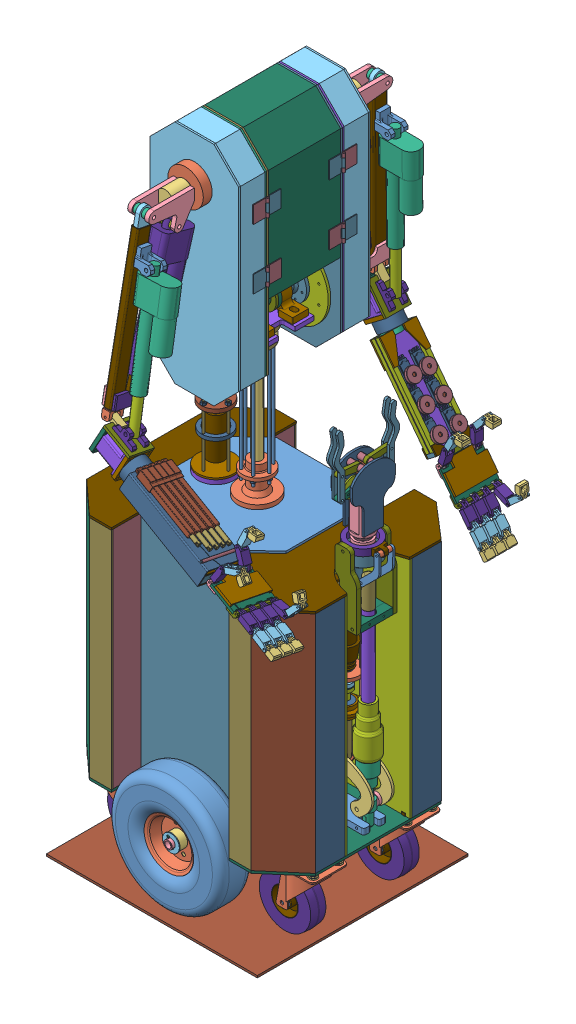
SolidWorks assembly sorbot, configuration По умолчанию. Lengths in mm. (continued)
Components (placement in the parent): (continued)
- finger.p2-17: finger.p2 [По умолчанию] at (252.1658 571.4308 -426.7503) x (0.604887 -0.796311 -0.000678) z (-0.005196 -0.004798 0.999975) size (48 12 20.5)
- finger.p3-11: finger.p3 [По умолчанию] at (275.7558 540.3742 -426.6638) x (0.604887 -0.796311 -0.000678) z (-0.005196 -0.004798 0.999975) size (30 12 20.5)
- finger.p1-12: finger.p1 [По умолчанию] at (225.5396 602.5263 -452.2401) x (0.917052 -0.398759 0.002852) z (-0.005196 -0.004798 0.999975) size (50 12 20.5)
- finger.p2-18: finger.p2 [По умолчанию] at (262.3245 581.0997 -452.1517) x (0.741393 0.671034 0.007072) z (-0.005196 -0.004798 0.999975) size (48 12 20.5)
- finger.p3-12: finger.p3 [По умолчанию] at (294.4266 604.5763 -451.7594) x (-0.075828 0.997111 0.00439) z (-0.005196 -0.004798 0.999975) size (30 12 20.5)
- bodu.tilit.axis.enforcement-1: bodu.tilit.axis.enforcement [По умолчанию] at (-20.0648 1016.5246 -221.0975) x (1 0 0) z (0 0 1) size (18 18 170.35)
- body_tilit_stud-5: body_tilit_stud [По умолчанию] at (-33.7006 648.7352 -112.3187) x (0.499707 0 -0.866195) z (0.866195 0 0.499707) size (6 307 6)
- body_tilit_stud-6: body_tilit_stud [По умолчанию] at (-5.5466 648.7352 -112.8281) x (-0.500293 0 -0.865856) z (0.865856 0 -0.500293) size (6 307 6)
- body_tilit_stud-7: body_tilit_stud [По умолчанию] at (8.0892 648.7352 -137.4649) x (-1 0 0.000338) z (-0.000338 0 -1) size (6 307 6)
- body_tilit_stud-8: body_tilit_stud [По умолчанию] at (-6.429 648.7352 -161.5923) x (-0.499707 0 0.866195) z (-0.866195 0 -0.499707) size (6 307 6)
- body_tilit_stud-9: body_tilit_stud [По умолчанию] at (-34.583 648.7352 -161.0828) x (0.500293 0 0.865856) z (-0.865856 0 0.500293) size (6 307 6)
- m6.nut-1: m6.nut [По умолчанию] at (8.0892 944.0246 -137.4649) size (10 5.5 11.55)
- m6.nut-2: m6.nut [По умолчанию] at (-6.429 944.0246 -161.5923) size (10 5.5 11.55)
- m6.nut-3: m6.nut [По умолчанию] at (-48.2188 944.0246 -136.446) size (10 5.5 11.55)
- m6.nut-4: m6.nut [По умолчанию] at (-34.583 944.0246 -161.0828) size (10 5.5 11.55)
- m6.nut-5: m6.nut [По умолчанию] at (-5.5466 944.0246 -112.8281) size (10 5.5 11.55)
- m6.nut-6: m6.nut [По умолчанию] at (-33.7006 944.0246 -112.3187) size (10 5.5 11.55)
- m6.nut-7: m6.nut [По умолчанию] at (-5.5466 657.2934 -112.8281) size (10 5.5 11.55)
- m6.nut-8: m6.nut [По умолчанию] at (-34.583 657.2934 -161.0828) size (10 5.5 11.55)
- m6.nut-9: m6.nut [По умолчанию] at (8.0892 657.2934 -137.4649) size (10 5.5 11.55)
- m6.nut-10: m6.nut [По умолчанию] at (-6.429 657.2934 -161.5923) size (10 5.5 11.55)
- m6.nut-11: m6.nut [По умолчанию] at (-33.7006 657.2934 -112.3187) size (10 5.5 11.55)
- m6.nut-12: m6.nut [По умолчанию] at (-48.2188 657.2934 -136.446) size (10 5.5 11.55)
- body.tilt.intermediate.enforce-1: body.tilt.intermediate.enforce [По умолчанию] at (-99.3474 976.856 -124.5942) x (1 0 0) z (0 1 0) size (30 25 30)
- arm.drive.p2-1: arm.drive.p2 [По умолчанию] at (43.6014 1241.2974 -35.5806) x (-0.089772 0 -0.995962) z (0.995962 0 -0.089772) size (134 5 24)
- arm.drive.p3-1: arm.drive.p3 [По умолчанию] at (3.7745 1243.7974 -50.7442) x (0 0 -1) z (0.174973 -0.984573 0) size (133.1 20 20)
- body.frame.p1-left-1: body.frame.p1-left [По умолчанию] at (-12.5682 795.4677 -226.3595) x (1 0 0) z (0 0 1) size (210 537.56 4)
- arm.drive.motor-1: arm.drive.motor [По умолчанию] at (-94.8762 1249.003 -67.2442) x (-0.533544 -0.845772 0) z (0.845772 -0.533544 0) size (117 39.5 152)
- arm.drive.motor.pair-1: arm.drive.motor.pair [По умолчанию] at (-76.8976 1162.9951 -205.8595) x (-0.885964 0.463755 0) z (0.463755 0.885964 0) size (117 39.5 152)
- arm.actuator.p2-5: arm.actuator.p2 [Default] at (-12.3884 1126.7783 -367.722) x (-0.005176 -0.088877 0.996029) z (0.999986 0 0.005196) size (20 180 20)
- arm.drive.p5-1: arm.drive.p5 [По умолчанию] at (3.7745 1243.7974 -58.7442) x (1 0 0) z (0 -1 0) size (34 8 34)
- arm.drive.p6-1: arm.drive.p6 [По умолчанию] at (3.7745 1243.7974 -50.7442) x (1 0 0) z (0 1 0) size (40 12 40)
- arm.drive.p3-2: arm.drive.p3 [По умолчанию] at (-20.8275 1162.0905 -222.3595) x (0 0 1) z (-0.923728 -0.383049 0) size (133.1 20 20)
- arm.drive.p5-2: arm.drive.p5 [По умолчанию] at (-20.8275 1162.0905 -214.3595) x (1 0 0) z (0 1 0) size (34 8 34)
- arm.drive.p6-2: arm.drive.p6 [По умолчанию] at (-20.8275 1162.0905 -222.3595) x (1 0.000029 0) z (0.000029 -1 0) size (40 12 40)
- arm.drive.p2-pair-1: arm.drive.p2-pair [По умолчанию] at (50.3811 1159.5904 -236.7848) x (-0.315418 0 0.948953) z (-0.948953 0 -0.315418) size (144 5 24)
- m14.nut-1: m14.nut [По умолчанию] at (-20.8275 1162.0905 -118.4852) x (0.513607 -0.858026 0) z (0.858026 0.513607 0) size (25.4 10.5 22.2)
- arm.drive.p7-2: arm.drive.p7 [По умолчанию] at (-14.5918 1147.0905 -123.4852) x (0 0 1) z (-1 0 0) size (28 15 59.47)
- arm.drive.p7-3: arm.drive.p7 [По умолчанию] at (-14.5918 1177.0905 -123.4852) x (0 0 -1) z (-1 0 0) size (28 15 59.47)
- arm.drive.p7-4: arm.drive.p7 [По умолчанию] at (10.1478 1228.9206 -145.3) x (0 0 1) z (-1 0 0) size (28 15 59.47)
- arm.drive.p7-5: arm.drive.p7 [По умолчанию] at (10.1478 1258.9206 -145.3) x (0 0 -1) z (-1 0 0) size (28 15 59.47)
- m14.nut-2: m14.nut [По умолчанию] at (3.7745 1243.7974 -150.3) x (-0.999875 0.015784 0) z (0.015784 0.999875 0) size (25.4 10.5 22.2)
- arm.drive.p1.m1-1: arm.drive.p1.m1 [По умолчанию] at (28.6519 1164.5905 -225.3595) x (0 1 0) z (-1 0 0) size (10 12 40)
- arm.drive.p1.m1-2: arm.drive.p1.m1 [По умолчанию] at (28.6519 1149.5905 -225.3595) x (0 1 0) z (-1 0 0) size (10 12 40)
- body.frame.p4.external-1: body.frame.p4.external [По умолчанию] at (-12.7111 795.3889 -292.3595) x (1 -0.000113 0) z (0 0 1) size (210 537.56 4)
- body.frame.p4.external-2: body.frame.p4.external [По умолчанию] at (-12.8242 795.3889 15.2558) x (1 -0.000113 0) z (0 0 1) size (210 537.56 4)
- arm.drive.p1.m1-3: arm.drive.p1.m1 [По умолчанию] at (65.4163 1231.2974 -47.7442) x (0 1 0) z (1 0 0) size (10 12 40)
- arm.drive.p1.m1-4: arm.drive.p1.m1 [По умолчанию] at (65.4163 1246.2974 -47.7442) x (0 1 0) z (1 0 0) size (10 12 40)
- body.frame.p4.right-1: body.frame.p4.right [По умолчанию] at (-12.4903 795.5195 -46.7442) x (1 0 0) z (0 0 1) size (210 537.56 4)
- arm.drive.p8-1: arm.drive.p8 [По умолчанию] at (-20.8275 1162.0905 -72.7442) x (-0.999995 0.003205 0) z (-0.003205 -0.999995 0) size (24 35.5 24)
- arm.drive.p8-2: arm.drive.p8 [По умолчанию] at (3.7745 1243.7974 -200.3595) x (1 0 0) z (0 -1 0) size (24 35.5 24)
- man1.drive1-1: man1.drive1 [По умолчанию] at (-118.5699 640.728 -137.5376) x (0.999934 0 -0.01146) z (0 1 0) size (50 50 148.25)
- body.tilit.planetary.drive.fixture.p1-1: body.tilit.planetary.drive.fixture.p1 [По умолчанию] at (-118.5699 612.7934 -137.5376) size (85 10 85)
- body.tilit.planetary.drive.fixture.p2-1: body.tilit.planetary.drive.fixture.p2 [По умолчанию] at (-118.5699 622.7934 -137.5376) size (85 4 85)
- tilt.thread.rod.fixture.2-2: tilt.thread.rod.fixture.2 [По умолчанию] at (-118.5699 793.5591 -137.5376) x (-0.837169 0 -0.546944) z (-0.546944 0 0.837169) size (40 26 40)
- body.tilit.planetary.drive.fixture.p3-1: body.tilit.planetary.drive.fixture.p3 [По умолчанию] at (-118.5699 695.728 -137.5376) size (68 8 68)
- body.tilit.planetary.drive.fixture.p4-1: body.tilit.planetary.drive.fixture.p4 [По умолчанию] at (-118.5699 753.9526 -137.5376) x (0.997546 0 -0.070011) z (0.070011 0 0.997546) size (70 9 70)
- body.tilit.planetary.drive.fixture.p5-1: body.tilit.planetary.drive.fixture.p5 [По умолчанию] at (-148.0595 612.7934 -137.5376) size (5 157 5)
- m6.nut-13: m6.nut [По умолчанию] at (-148.0595 613.2934 -137.5376) size (10 5.5 11.55)
- body.tilit.planetary.drive.fixture.p5-2: body.tilit.planetary.drive.fixture.p5 [По умолчанию] at (-89.0803 612.7934 -137.5376) size (5 157 5)
- body.tilit.planetary.drive.fixture.p5-3: body.tilit.planetary.drive.fixture.p5 [По умолчанию] at (-118.5699 612.7934 -108.048) size (5 157 5)
- body.tilit.planetary.drive.fixture.p5-4: body.tilit.planetary.drive.fixture.p5 [По умолчанию] at (-118.5699 612.7934 -167.0272) size (5 157 5)
- m6.nut-14: m6.nut [По умолчанию] at (-89.0803 613.2934 -137.5376) size (10 5.5 11.55)
- m6.nut-15: m6.nut [По умолчанию] at (-118.5699 613.2934 -167.0272) x (0.598875 0 -0.800843) z (0.800843 0 0.598875) size (10 5.5 11.55)
- m6.nut-16: m6.nut [По умолчанию] at (-118.5699 613.2934 -108.048) x (-0.286054 0 -0.958214) z (0.958214 0 -0.286054) size (10 5.5 11.55)
- m6.nut-17: m6.nut [По умолчанию] at (-118.5699 768.4526 -108.048) x (-0.837169 0 -0.546944) z (-0.546944 0 0.837169) size (10 5.5 11.55)
- m6.nut-18: m6.nut [По умолчанию] at (-89.0803 768.4526 -137.5376) x (-0.837169 0 -0.546944) z (-0.546944 0 0.837169) size (10 5.5 11.55)
- m6.nut-19: m6.nut [По умолчанию] at (-118.5699 768.4526 -167.0272) x (-0.837169 0 -0.546944) z (-0.546944 0 0.837169) size (10 5.5 11.55)
- m6.nut-20: m6.nut [По умолчанию] at (-148.0595 768.4526 -137.5376) x (-0.837169 0 -0.546944) z (-0.546944 0 0.837169) size (10 5.5 11.55)
- m6.nut-21: m6.nut [По умолчанию] at (-29.5996 1324.99 9.9014) x (-0.526603 0.850111 0) z (0 0 1) size (10 5.5 11.55)
- m6.6.50mm-1: m6.6.50mm [По умолчанию] at (4.3029 1345.9909 9.9014) x (0.525089 -0.847668 0.075763) z (-0.039897 0.064407 0.997126) size (10 56 10)
- m4.nut-1: m4.nut [По умолчанию] at (-35.3987 1340.8364 4.6679) x (1 0 0) z (0 -1 0) size (6.86 5 7.92)
- m4.nut-2: m4.nut [По умолчанию] at (-103.2224 997.8992 -35.7442) x (1 0 0) z (0 -1 0) size (6.86 5 7.92)
Mates (geometry in assembly coordinates):
- Концентричный1: concentric anti-aligned: cylinder of wheel-2/wheel.metal.internal-1 through (-6.6918 11.9368 -351.3681) axis (0 0 1) radius 10; cylinder of wheel-1/wheel.metal.internal-1 through (-6.6918 11.9368 79.1319) axis (0 0 -1) radius 10
- Концентричный2: concentric anti-aligned: cylinder of wheel-1/wheel.metal.internal-1 through (-6.6918 11.9368 79.1319) axis (0 0 -1) radius 10; cylinder of wheel.axis-1 through (-6.6918 11.9368 -361.8681) axis (0 0 1) radius 10
- Концентричный3: concentric anti-aligned: cylinder of wheel.axis-1 through (-6.6918 11.9368 -361.8681) axis (0 0 1) radius 10; cylinder of wheel.washer-1 through (-6.6918 11.9368 81.1319) axis (0 0 -1) radius 10
- Совпадение3: coincident anti-aligned: plane of wheel-1/wheel.metal.internal-1 through (-6.6918 11.9368 79.1319) normal (0 0 1); plane of wheel.washer-1 through (-6.6918 11.9368 79.1319) normal (0 0 -1)
- Концентричный4: concentric anti-aligned: cylinder of wheel.axis-1 through (-6.6918 11.9368 -361.8681) axis (0 0 1) radius 10; cylinder of wheel.washer-2 through (-6.6918 11.9368 -351.3681) axis (0 0 -1) radius 10
- Совпадение4: coincident anti-aligned: plane of wheel.washer-2 through (-6.6918 11.9368 -351.3681) normal (0 0 1); plane of wheel-2/wheel.metal.internal-1 through (-6.6918 11.9368 -351.3681) normal (0 0 -1)
- Параллельность1: parallel aligned: cylinder of wheel.axis-1 through (0.9691 -6.5378 -355.8681) axis (-0.383049 0.923728 0) radius 1; line of wheel.axis.splint-2 through (-3.0707 5.7105 -356.5951) axis (-0.383049 0.923728 0)
- Концентричный5: concentric aligned: cylinder of wheel-2/wheel.metal.internal-1 through (-6.6918 11.9368 -291.3681) axis (0 0 -1) radius 19; cylinder of wheel.disk-1 through (-6.6918 11.9368 -311.3681) axis (0 0 -1) radius 18.9
- Совпадение7: coincident anti-aligned: plane of wheel-2/wheel.metal.internal-1 through (-25.4032 15.2361 -326.3681) normal (0 0 1); plane of wheel.disk-1 through (-6.6918 11.9368 -326.3681) normal (0 0 -1)
- Концентричный6: concentric anti-aligned: cylinder of wheel.axis-1 through (-6.6918 11.9368 -361.8681) axis (0 0 1) radius 10; cylinder of wheel.bearing-1 through (-6.6918 11.9368 -256.3681) axis (0 0 -1) radius 10
- Концентричный8: concentric aligned: cylinder of wheel.axis-1 through (-6.6918 11.9368 -361.8681) axis (0 0 1) radius 10; cylinder of wheel.stop.bearing-2/wheel.stop.bearing.p1-2 through (-6.6918 11.9368 -246.3457) axis (0 0 1) radius 10
- Совпадение10: coincident anti-aligned: plane of wheel.disk-1 through (-6.6918 11.9368 -256.3681) normal (0 0 1); plane of wheel.stop.bearing-2/wheel.stop.bearing.p1-1 through (-6.6918 11.9368 -256.3681) normal (0 0 -1)
- Концентричный10: concentric anti-aligned: cylinder of gearmotor-1 through (53.2168 119.2767 -284.0001) axis (0 0 1) radius 7; cylinder of gearmotor.sprocket.wheel.disk-1 through (53.2168 119.2767 -217.7117) axis (0 0 -1) radius 7
- Концентричный13: concentric anti-aligned: cylinder of wheel.axis-1 through (-6.6918 11.9368 -361.8681) axis (0 0 1) radius 10; cylinder of sprocket-1 through (-6.6918 11.9368 -268.3681) axis (0 0 -1) radius 26
- Концентричный14: concentric anti-aligned: circle of gearmotor-1; circle of sproket.initial-1
- Совпадение16: coincident aligned: plane of sproket.initial-1 through (64.3825 152.5534 -268.5001) normal (0 0 1); circle of gearmotor.sprocket.wheel.disk-1
- Параллельность2: parallel anti-aligned: plane of sproket.initial-1 through (64.3825 152.5534 -271.5001) normal (0 0 -1); plane of sprocket-1 through (4.6992 45.137 -268.3681) normal (0 0 1)
- Совпадение57: coincident anti-aligned: plane of sprocket-1 through (4.6992 45.137 -271.3681) normal (0 0 -1); plane of wheel.disk-1 through (-6.6918 11.9368 -271.3681) normal (0 0 1)
- Совпадение61: coincident anti-aligned: plane of gearmotor-1 through (53.2168 119.2767 -254.0001) normal (0 0 -1); plane of gearmotor.sprocket.wheel.disk-1 through (53.2168 119.2767 -254.0001) normal (0 0 1)
- Параллельность3: parallel aligned: plane of sproket.initial-1 through (64.3825 152.5534 -268.5001) normal (0 0 1); plane of sprocket-1 through (4.6992 45.137 -268.3681) normal (0 0 1)
- Совпадение65: coincident anti-aligned: plane of bottom-2 through (-49.3372 46.4368 -286.1821) normal (0 -1 0); plane of wheel.axis.frame-3 through (15.3082 46.4368 -205.8457) normal (0 1 0)
- Концентричный59: concentric anti-aligned: cylinder of wheel.axis-1 through (-6.6918 11.9368 -361.8681) axis (0 0 1) radius 10; cylinder of wheel.axis.frame-3 through (-6.6918 11.9368 -211.3457) axis (0 0 -1) radius 10
- Совпадение66: coincident anti-aligned: plane of wheel.stop.bearing-2/wheel.stop.bearing.p1-2 through (-6.6918 11.9368 -242.3457) normal (0 0 1); plane of wheel.axis.frame-3 through (-6.6918 11.9368 -242.3457) normal (0 0 -1)
- Совпадение68: coincident anti-aligned: plane of wheel.disk-2 through (-6.6918 11.9368 54.1319) normal (0 0 1); plane of wheel-1/wheel.metal.internal-1 through (11.3638 17.8524 54.1319) normal (0 0 -1)
- Концентричный60: concentric aligned: cylinder of wheel-1/wheel.metal.internal-1 through (-6.6918 11.9368 19.1319) axis (0 0 1) radius 19; cylinder of wheel.disk-2 through (-6.6918 11.9368 39.1319) axis (0 0 1) radius 18.9
- Концентричный62: concentric anti-aligned: cylinder of wheel.axis-1 through (-6.6918 11.9368 -361.8681) axis (0 0 1) radius 10; cylinder of wheel.bearing-2 through (-6.6918 11.9368 -8.8681) axis (0 0 -1) radius 10
- Совпадение69: coincident anti-aligned: plane of wheel.disk-2 through (-6.6918 11.9368 -8.8681) normal (0 0 -1); plane of wheel.bearing-2 through (-6.6918 11.9368 -8.8681) normal (0 0 1)
- Концентричный63: concentric aligned: cylinder of wheel.axis-1 through (-6.6918 11.9368 -361.8681) axis (0 0 1) radius 10; cylinder of wheel.stop.bearing-3/wheel.stop.bearing.p1-2 through (-6.6918 11.9368 -19.8681) axis (0 0 1) radius 10
- Совпадение70: coincident anti-aligned: plane of wheel.bearing-2 through (-6.6918 11.9368 -15.8681) normal (0 0 -1); plane of wheel.stop.bearing-3/wheel.stop.bearing.p1-2 through (-6.6918 11.9368 -15.8681) normal (0 0 1)
- Совпадение72: coincident anti-aligned: plane of wheel.axis.frame-4 through (-28.6918 46.4368 -66.3906) normal (0 1 0); plane of bottom-2 through (-49.3372 46.4368 -286.1821) normal (0 -1 0)
- Совпадение73: coincident anti-aligned: plane of wheel.axis.frame-4 through (-6.6918 11.9368 -29.8906) normal (0 0 1); plane of wheel.stop.bearing-3/wheel.stop.bearing.p1-1 through (-6.6918 11.9368 -29.8906) normal (0 0 -1)
- Концентричный65: concentric aligned: cylinder of wheel.axis-1 through (-6.6918 11.9368 -361.8681) axis (0 0 1) radius 10; cylinder of wheel.axis.frame-4 through (-6.6918 11.9368 -60.8906) axis (0 0 1) radius 10
- Совпадение74: coincident anti-aligned: plane of wheel.disk-2 through (-6.6918 11.9368 -0.8681) normal (0 0 -1); plane of sprocket-2 through (4.3334 45.2603 -0.8681) normal (0 0 1)
- Концентричный66: concentric anti-aligned: cylinder of wheel.disk-2 through (-6.6918 11.9368 -15.8681) axis (0 0 1) radius 26.5; cylinder of sprocket-2 through (-6.6918 11.9368 -0.8681) axis (0 0 -1) radius 26
- Концентричный67: concentric anti-aligned: cylinder of gearmotor-2 through (-40.8776 119.0545 10.8308) axis (0 0 -1) radius 7; cylinder of gearmotor.sprocket.wheel.disk-2 through (-40.8776 119.0545 -55.4577) axis (0 0 1) radius 7
- Совпадение77: coincident anti-aligned: plane of gearmotor.sprocket.wheel.disk-2 through (-40.8776 119.0545 -19.1692) normal (0 0 -1); plane of gearmotor-2 through (-40.8776 119.0545 -19.1692) normal (0 0 1)
- Совпадение78: coincident anti-aligned: plane of gearmotor-2 through (-39.033 127.9382 4.8308) normal (0.999846 0.017524 0); plane of gearmotor.sprocket.wheel.disk-2 through (-39.033 127.9382 -55.4577) normal (-0.999846 -0.017524 0)
- Совпадение79: coincident anti-aligned: plane of sproket.initial-2 through (-52.3821 152.2156 -4.6692) normal (0 0 -1); plane of gearmotor.sprocket.wheel.disk-2 through (-40.8776 119.0545 -4.6692) normal (0 0 1)
- Концентричный68: concentric anti-aligned: circle of gearmotor.sprocket.wheel.disk-2; circle of sproket.initial-2
- Концентричный69: concentric aligned: cylinder of wheel.axis-1 through (-6.6918 11.9368 -361.8681) axis (0 0 1) radius 10; cylinder of wheel.disk-2 through (-6.6918 11.9368 39.1319) axis (0 0 1) radius 18.9
- Заблокировать1: lock: unknown of ?; unknown of ?
- Заблокировать3: lock: unknown of ?; unknown of ?
- Заблокировать4: lock: unknown of ?; unknown of ?
- Совпадение81: coincident anti-aligned: plane of wheel.disk-1 through (-6.6918 11.9368 -263.3681) normal (0 0 1); plane of wheel.bearing-1 through (-6.6918 11.9368 -263.3681) normal (0 0 -1)
- Концентричный77: concentric anti-aligned: cylinder of gearmotor-2 through (-40.8776 119.0545 -257.1692) axis (0 0 1) radius 32.5; cylinder of gearmotor.fixture.p3-1 through (-40.8776 119.0545 -181.1702) axis (0 0 -1) radius 32.4
- Концентричный80: concentric anti-aligned: cylinder of gearmotor-1 through (53.2168 119.2767 -250.0001) axis (0 0 1) radius 20; cylinder of gearmotor.fixture.p2-3 through (53.2168 119.2767 -237.0001) axis (0 0 -1) radius 21.5
- Совпадение104: coincident anti-aligned: plane of gearmotor-1 through (53.2168 119.2767 -245.0001) normal (0 0 -1); plane of gearmotor.fixture.p2-3 through (10.2084 53.4933 -245.0001) normal (0 0 1)
- Параллельность25: parallel aligned: line of bottom-2 through (267.1742 51.9368 11.9714) axis (0 0 -1); line of wall1-1 through (26.1889 166.4368 -62.2424) axis (0 0 -1)
- Совпадение111: coincident aligned: line of wall1-1 through (21.1889 585.1505 -212.2424) axis (0 -1 0); line of wall2-2 through (21.1889 585.1505 -212.2424) axis (0 -1 0)
- Совпадение114: coincident anti-aligned: plane of wall2-2 through (21.1889 831.1682 -212.2424) normal (0 0 1); plane of wall3-1 through (107.1741 171.4368 -212.2424) normal (0 0 -1)
- Совпадение116: coincident aligned: line of wall2-2 through (107.1741 51.9368 -216.2424) axis (0 1 0); line of wall4-1 through (107.1741 51.4368 -216.2424) axis (0 1 0)
- Совпадение117: coincident anti-aligned: plane of wall2-2 through (107.1741 -108.1132 -212.2424) normal (-1 0 0); plane of wall4-1 through (107.1741 51.4368 -56.2424) normal (1 0 0)
- Совпадение120: coincident anti-aligned: plane of wall2-1 through (21.1889 831.1682 -58.2424) normal (0 0 1); plane of wall6-1 through (263.1742 655.3334 -58.2424) normal (0 0 -1)
- Совпадение121: coincident anti-aligned: plane of bottom-2 through (-49.3372 51.9368 -286.1821) normal (0 1 0); plane of wall6-1 through (263.1742 51.9368 -58.2424) normal (0 -1 0)
- Совпадение122: coincident aligned: line of bottom-2 through (267.1742 51.9368 11.9714) axis (0 0 -1); line of wall6-1 through (267.1742 51.9368 11.8264) axis (0 0 -1)
- Параллельность26: parallel aligned: line of bottom-2 through (184.9009 51.9368 82.4522) axis (0.759435 0 -0.650583); line of wall7-1 through (184.8921 51.9368 82.4377) axis (0.759435 0 -0.650583)
- Совпадение127: coincident anti-aligned: plane of bottom-2 through (-49.3372 51.9368 -286.1821) normal (0 1 0); plane of wall7-1 through (263.5537 51.9368 9.7838) normal (0 -1 0)
- Совпадение131: coincident anti-aligned: line of bottom-2 through (267.1742 51.9368 11.9714) axis (0 0 -1); line of wall6-3 through (267.1742 51.9368 -286.3112) axis (0 0 1)
- Совпадение132: coincident anti-aligned: line of wall6-3 through (267.1742 51.9368 -216.2424) axis (0 1 0); line of wall2-2 through (267.1741 585.1505 -216.2424) axis (0 -1 0)
- Совпадение136: coincident aligned: line of bottom-2 through (132.9009 51.9368 12.4522) axis (0 0 1); line of wall8-1 through (132.9009 51.9368 78.4522) axis (0 0 1)
- Совпадение137: coincident aligned: line of bottom-2 through (132.9009 51.9368 82.4522) axis (1 0 0); line of wall8-1 through (132.9009 51.9368 82.4522) axis (1 0 0)
- Совпадение142: coincident anti-aligned: plane of bottom-2 through (-49.3372 51.9368 -286.1821) normal (0 1 0); plane of wall8-2 through (141.3107 51.9368 -178.9033) normal (0 -1 0)
- Совпадение143: coincident anti-aligned: plane of wall8-1 through (132.9009 637.4067 78.4522) normal (0 0 -1); plane of wall9-1 through (132.9009 655.1671 78.4522) normal (0 0 1)
- Совпадение144: coincident anti-aligned: plane of bottom-2 through (-49.3372 51.9368 -286.1821) normal (0 1 0); plane of wall9-1 through (132.9009 51.9368 78.4522) normal (0 -1 0)
- Совпадение145: coincident aligned: line of bottom-2 through (132.9009 51.9368 12.4522) axis (0 0 1); line of wall9-1 through (132.9009 51.9368 8.55) axis (0 0 1)
- Совпадение146: coincident aligned: line of bottom-2 through (39.4201 51.9368 12.4522) axis (1 0 0); line of wall10-1 through (-146.6756 51.9368 12.4522) axis (1 0 0)
- Совпадение147: coincident anti-aligned: plane of wall9-1 through (132.9009 655.1671 8.55) normal (-1 0 0); plane of wall10-1 through (132.9009 864.7556 8.4522) normal (1 0 0)
- Совпадение149: coincident anti-aligned: plane of bottom-2 through (-49.3372 51.9368 -286.1821) normal (0 1 0); plane of wall9-2 through (-150.6756 51.9368 78.5322) normal (0 -1 0)
- Совпадение157: coincident anti-aligned: line of wall3-1 through (107.1741 166.4368 -62.2424) axis (0 0 -1); line of wall4-1 through (107.1741 166.4368 -216.2424) axis (0 0 1)
- Совпадение161: coincident anti-aligned: line of wall2-2 through (21.1889 166.4368 -212.2424) axis (1 0 0); line of wall3-1 through (107.1741 166.4368 -212.2424) axis (-1 0 0)
- Совпадение162: coincident anti-aligned: line of wall2-1 through (107.1741 166.4368 -62.2424) axis (-1 0 0); line of wall3-1 through (26.1889 166.4368 -62.2424) axis (1 0 0)
- Совпадение170: coincident anti-aligned: plane of bottom-2 through (-49.3372 51.9368 -286.1821) normal (0 1 0); plane of wall7-v1-1 through (-149.98 51.9368 -93.7194) normal (0 -1 0)
- Параллельность29: parallel anti-aligned: line of bottom-2 through (-275.9596 51.9368 11.9714) axis (0.73854 0 0.67421); line of wall7-v1-1 through (-199.0366 51.9368 82.0998) axis (-0.73854 0 -0.67421)
- Совпадение174: coincident anti-aligned: line of wall7-v1-1 through (-275.9003 51.9368 11.9312) axis (0 1 0); line of wall11-1 through (-275.9003 585.1505 11.9312) axis (0 -1 0)
- Совпадение180: coincident anti-aligned: line of wall7-v1-2 through (-198.8179 51.9368 -356.1236) axis (0 1 0); line of wall8-5 through (-198.8179 585.1505 -356.1236) axis (0 -1 0)
- Совпадение181: coincident anti-aligned: plane of bottom-2 through (-49.3372 51.9368 -286.1821) normal (0 1 0); plane of wall8-5 through (-146.715 51.9368 -356.1236) normal (0 -1 0)
- Параллельность31: parallel aligned: line of bottom-2 through (-146.7539 51.9368 -356.1821) axis (-1 0 0); line of wall8-5 through (-146.715 51.9368 -356.1236) axis (-1 0 0)
- Совпадение182: coincident anti-aligned: plane of bottom-2 through (-49.3372 51.9368 -286.1821) normal (0 1 0); plane of wall9-3 through (-150.8245 51.9368 -282.1286) normal (0 -1 0)
- Совпадение184: coincident anti-aligned: plane of bottom-2 through (-49.3372 51.9368 -286.1821) normal (0 1 0); plane of wall10-v1-1 through (132.7521 51.9368 -286.1286) normal (0 -1 0)
- Совпадение187: coincident aligned: line of wall9-3 through (-146.8245 585.1505 -282.1286) axis (0 -1 0); line of wall10-v1-1 through (-146.8245 585.1505 -282.1286) axis (0 -1 0)
- Совпадение188: coincident anti-aligned: plane of bottom-2 through (-49.3372 51.9368 -286.1821) normal (0 1 0); plane of wall9-4 through (132.7521 51.9368 -282.1286) normal (0 -1 0)
- Совпадение189: coincident aligned: line of wall10-v1-1 through (132.7521 585.1505 -282.1286) axis (0 -1 0); line of wall9-4 through (132.7521 585.1505 -282.1286) axis (0 -1 0)
- Совпадение191: coincident anti-aligned: line of bottom-2 through (184.9009 51.9368 -356.1821) axis (-1 0 0); line of wall8-2 through (132.798 51.9368 -356.1821) axis (1 0 0)
- Совпадение201: coincident anti-aligned: plane of bottom-2 through (-49.3372 51.9368 -286.1821) normal (0 1 0); plane of wall7-3 through (183.3311 51.9368 -352.2595) normal (0 -1 0)
- Параллельность33: parallel aligned: line of bottom-2 through (267.1742 51.9368 -285.7013) axis (-0.759435 0 -0.650583); line of wall7-3 through (267.1973 51.9368 -285.6811) axis (-0.759435 0 -0.650583)
- Параллельность52: parallel anti-aligned: plane of gearmotor-3 through (-22.0648 623.1505 -128.1055) normal (-1 0 0); plane of turret-1/turret-p1-1 through (-22.0648 627.1934 -130.2473) normal (1 0 0)
- Концентричный93: concentric aligned: cylinder of gearmotor-3 through (-20.0648 629.1505 -136.9555) axis (0 -1 0) radius 7; cylinder of turret-1/turret-p1-1 through (-20.0648 627.1934 -136.9555) axis (0 -1 0) radius 7
- Концентричный110: concentric anti-aligned: cylinder of bolt1-2 through (172.9115 63.0264 3.3236) axis (0 -1 0) radius 5; cylinder of bolt1.nut-9 through (172.9115 51.9368 3.3236) axis (0 1 0) radius 5
- Концентричный111: concentric anti-aligned: cylinder of turret-1/turret-p1-1 through (-20.0648 603.2934 -136.9555) axis (0 1 0) radius 74; cylinder of turret.table-1 through (-20.0648 612.7934 -136.9555) axis (0 -1 0) radius 35
- Концентричный112: concentric aligned: cylinder of gearmotor-3 through (-20.0648 629.1505 -136.9555) axis (0 -1 0) radius 7; cylinder of ? through (-20.0648 622.7934 -136.9555) axis (0 -1 0) radius 7
- Совпадение223: coincident anti-aligned: plane of turret-1/turret-p1-1 through (-20.0648 607.7934 -136.9555) normal (0 1 0); plane of ? through (-20.0648 607.7934 -136.9555) normal (0 -1 0)
- Совпадение230: coincident anti-aligned: plane of gearmotor.fixture.p2-3 through (10.2084 53.4933 -245.0001) normal (0 1 0); plane of wheel.axis.frame.fixture.p2-3 through (-51.698 53.4933 -213.5833) normal (0 -1 0)
- Совпадение236: coincident anti-aligned: plane of bottom-2 through (-49.3372 51.9368 -286.1821) normal (0 1 0); plane of wall-fixture-3-2 through (213.2226 51.9368 -31.5478) normal (0 -1 0)
- Совпадение242: coincident anti-aligned: plane of gearmotor-2 through (-40.8776 119.0545 -28.1692) normal (0 0 1); plane of gearmotor.fixture.p2.1-1 through (2.1309 53.4368 -28.1692) normal (0 0 -1)
- Совпадение246: coincident anti-aligned: plane of bottom-2 through (-49.3372 51.9368 -286.1821) normal (0 1 0); plane of wheel.axis.frame.fixture.p2-1 through (43.2929 51.9368 -36.1421) normal (0 -1 0)
- Совпадение248: coincident anti-aligned: plane of wheel.axis.frame-4 through (15.3082 32.4368 -66.3906) normal (0 -1 0); plane of wheel.axis.frame.fixture.p1-1 through (42.6901 32.4368 -36.0198) normal (0 1 0)
- Концентричный116: concentric aligned: circle of wheel.axis.frame.fixture.p1-1; circle of wheel.axis.frame.fixture.p2-1
- Совпадение252: coincident anti-aligned: plane of wall7-v1-1 through (-271.8817 585.1505 10.1837) normal (0 1 0); plane of cap-1 through (216.6954 585.1505 -83.7838) normal (0 -1 0)
- Совпадение253: coincident anti-aligned: plane of cap-1 through (216.6954 590.1505 -83.7838) normal (0 1 0); plane of turret-1/turret-p4-1 through (-19.4709 590.1505 -137.0226) normal (0 -1 0)
- Совпадение254: coincident anti-aligned: plane of turret-1/turret-p1-1 through (-20.0648 607.7934 -136.9555) normal (0 1 0); plane of turret.table-1 through (-21.0698 607.7934 -363.9712) normal (0 -1 0)
- Заблокировать30: lock: unknown of ?; unknown of ?
- Заблокировать31: lock: unknown of ?; unknown of ?
- Заблокировать32: lock: unknown of ?; unknown of ?
- Заблокировать33: lock: unknown of ?; unknown of ?
- Заблокировать34: lock: unknown of ?; unknown of ?
- Заблокировать35: lock: unknown of ?; unknown of ?
- Заблокировать36: lock: unknown of ?; unknown of ?
- Заблокировать37: lock: unknown of ?; unknown of ?
- Заблокировать38: lock: unknown of ?; unknown of ?
- Заблокировать39: lock: unknown of ?; unknown of ?
- Заблокировать40: lock: unknown of ?; unknown of ?
- Заблокировать41: lock: unknown of ?; unknown of ?
- Совпадение276: coincident anti-aligned: plane of bottom-2 through (-49.3372 51.9368 -286.1821) normal (0 1 0); plane of wall-fixture-3-3-1 through (-242.5877 51.9368 -17.2349) normal (0 -1 0)
- Совпадение277: coincident anti-aligned: plane of wall7-v1-1 through (-271.8817 -52.2153 10.1837) normal (0.67421 0 -0.73854); plane of wall-fixture-3-3-1 through (-269.5561 51.9368 12.3067) normal (-0.67421 0 0.73854)
- Заблокировать42: lock: unknown of ?; unknown of ?
- Заблокировать43: lock: unknown of ?; unknown of ?
- Заблокировать44: lock: unknown of ?; unknown of ?
- Заблокировать45: lock: unknown of ?; unknown of ?
- Заблокировать46: lock: unknown of ?; unknown of ?
- Заблокировать47: lock: unknown of ?; unknown of ?
- Заблокировать48: lock: unknown of ?; unknown of ?
- Заблокировать49: lock: unknown of ?; unknown of ?
- Заблокировать50: lock: unknown of ?; unknown of ?
- Заблокировать51: lock: unknown of ?; unknown of ?
- Заблокировать52: lock: unknown of ?; unknown of ?
- Заблокировать53: lock: unknown of ?; unknown of ?
- Совпадение282: coincident anti-aligned: plane of bottom-2 through (-49.3372 51.9368 -286.1821) normal (0 1 0); plane of bolt1.nut-1 through (-189.5596 51.9368 -278.9161) normal (0 -1 0)
- Заблокировать54: lock: unknown of ?; unknown of ?
- Заблокировать55: lock: unknown of ?; unknown of ?
- Заблокировать56: lock: unknown of ?; unknown of ?
- Заблокировать57: lock: unknown of ?; unknown of ?
- Заблокировать58: lock: unknown of ?; unknown of ?
- Заблокировать59: lock: unknown of ?; unknown of ?
- Заблокировать60: lock: unknown of ?; unknown of ?
- Заблокировать61: lock: unknown of ?; unknown of ?
- Заблокировать62: lock: unknown of ?; unknown of ?
- Заблокировать63: lock: unknown of ?; unknown of ?
- Заблокировать64: lock: unknown of ?; unknown of ?
- Заблокировать65: lock: unknown of ?; unknown of ?
- Совпадение287: coincident anti-aligned: plane of bottom-2 through (-49.3372 51.9368 -286.1821) normal (0 1 0); plane of bolt1.nut-9 through (180.9944 51.9368 3.3236) normal (0 -1 0)
- Заблокировать66: lock: unknown of ?; unknown of ?
- Заблокировать67: lock: unknown of ?; unknown of ?
- Заблокировать68: lock: unknown of ?; unknown of ?
- Заблокировать69: lock: unknown of ?; unknown of ?
- Заблокировать70: lock: unknown of ?; unknown of ?
- Заблокировать71: lock: unknown of ?; unknown of ?
- Заблокировать72: lock: unknown of ?; unknown of ?
- Заблокировать73: lock: unknown of ?; unknown of ?
- Заблокировать75: lock: unknown of ?; unknown of ?
- Заблокировать76: lock: unknown of ?; unknown of ?
- Заблокировать77: lock: unknown of ?; unknown of ?
- Совпадение290: coincident anti-aligned: plane of bottom-2 through (-49.3372 51.9368 -286.1821) normal (0 1 0); plane of bolt1.nut-13 through (164.6729 51.9368 -277.7529) normal (0 -1 0)
- Касательный1: tangent anti-aligned: cylinder of wheel-1/wheel.chamber-1 through (-6.6918 11.9368 97.7637) axis (0 0 -1) radius 135; plane of ground-1 through (232.7402 -123.0632 115.6816) normal (0 1 0)
- Концентричный125: concentric aligned: cylinder of body.center-1 through (-20.0648 982.0246 -136.9555) axis (0 -1 0) radius 11; cylinder of body_pivot_fixture-1 through (-20.0648 962.0246 -136.9555) axis (0 -1 0) radius 11
- Совпадение298: coincident anti-aligned: plane of turret.table-1 through (-21.0698 612.7934 -363.9712) normal (0 1 0); plane of body_tilt_drive_frame_p1-1 through (-114.5094 612.7934 -273.8211) normal (0 -1 0)
- Совпадение299: coincident: point of turret.table-1; unknown of body_tilt_drive_frame_p1-1
- Совпадение300: coincident: unknown of turret.table-1; unknown of body_tilt_drive_frame_p1-2
- Совпадение301: coincident anti-aligned: plane of turret.table-1 through (-21.0698 612.7934 -363.9712) normal (0 1 0); plane of body_tilt_drive_frame_p1-2 through (72.3667 612.7934 -1.7032) normal (0 -1 0)
- Совпадение315: coincident aligned: line of turret.table-1 through (-173.1373 612.7934 -54.2032) axis (0.72933 0 0.684163); line of body_tilt_drive_frame_p2-1 through (-173.1373 612.7934 -54.2032) axis (0.72933 0 0.684163)
- Концентричный163: concentric aligned: cylinder of body_axis-1 through (-20.0648 1016.5246 -50.7475) axis (0 0 -1) radius 10.9; cylinder of body.frame.p1.fixture-2 through (-20.0648 1016.5246 -209.3595) axis (0 0 -1) radius 10.9
- Заблокировать91: lock: unknown of ?; unknown of ?
- Параллельность60: parallel aligned: cylinder of arm.actuator-1/arm.actuator.p1-1 through (-88.5767 993.1387 1.2558) axis (0 0 -1) radius 4.1; cylinder of arm.actuator.p2-1 through (-61.0144 1401.6056 11.2558) axis (0 0 -1) radius 4
- Концентричный165: concentric anti-aligned: cylinder of arm.actuator-1/arm.actuator.p1-1 through (-79.5552 1126.8347 -13.7442) axis (0.067324 0.997731 0) radius 10; cylinder of arm.actuator.p2-1 through (-60.4422 1410.0864 -13.7442) axis (-0.067324 -0.997731 0) radius 10
- Концентричный454: concentric: cylinder of arm.actuator-1/arm.actuator.p1-1 through (-88.5767 993.1387 1.2558) axis (0 0 -1) radius 4.1; cylinder of arm.lift.actuator.fixture.p2-1 through (-88.5767 993.1387 15.1693) axis (0 0 -1) radius 4
- Касательный32: tangent anti-aligned: cylinder of arm.actuator-1/arm.actuator.p1-1 through (-89.1153 985.1568 -13.7442) axis (0.067324 0.997731 0) radius 10; plane of arm.lift.actuator.fixture.p3-1 through (-88.5767 993.1387 -3.7442) normal (0 0 -1)
- Концентричный176: concentric aligned: cylinder of arm.actuator.p2-1 through (-61.0144 1401.6056 11.2558) axis (0 0 -1) radius 4; cylinder of shoulder.p4-1 through (-61.0144 1401.6056 -23.7442) axis (0 0 -1) radius 4
- Концентричный179: concentric aligned: cylinder of arm.actuator.p2-1 through (-61.0144 1401.6056 11.2558) axis (0 0 -1) radius 4; cylinder of ? through (-61.0144 1401.6056 0.2558) axis (0 0 -1) radius 4
- Концентричный183: concentric aligned: cylinder of arm.lift.actuator.fixture.p2-1 through (-88.5767 993.1387 15.1693) axis (0 0 -1) radius 4; cylinder of arm.lift.actuator.fixture.p3-1 through (-88.5767 993.1387 15.2558) axis (0 0 -1) radius 4
- Касательный11: tangent anti-aligned: cylinder of arm.actuator.p2-1 through (-60.4422 1410.0864 -13.7442) axis (-0.067324 -0.997731 0) radius 10; plane of ? through (-59.9468 1400.1462 -3.7442) normal (0 0 -1)
- Касательный12: tangent anti-aligned: cylinder of arm.actuator.p2-1 through (-60.4422 1410.0864 -13.7442) axis (-0.067324 -0.997731 0) radius 10; plane of shoulder.p4-1 through (-59.9469 1400.1462 -23.7442) normal (0 0 1)
- Заблокировать105: lock: unknown of ?; unknown of ?
- Заблокировать106: lock: unknown of ?; unknown of ?
- Концентричный203: concentric anti-aligned: cylinder of arm.actuator-2/arm.actuator.p1-1 through (-12.7848 1158.0223 117.7054) axis (0 -0.960187 0.279359) radius 10; cylinder of arm.actuator.p2-2 through (-12.7848 966.8747 173.3183) axis (0 0.960187 -0.279359) radius 10
- Концентричный217: concentric anti-aligned: cylinder of arm.actuator100mm.p2-1 through (40.0811 939.5824 217.2691) axis (-0.032442 0.981084 -0.190842) radius 10; cylinder of arm.actuator100mm..p1-1 through (32.6076 1165.5904 173.3056) axis (0.032442 -0.981084 0.190842) radius 10
- Параллельность77: parallel anti-aligned: cylinder of arm.actuator100mm..p1-1 through (29.8176 1247.0995 142.1691) axis (0 0.190943 0.981601) radius 4; cylinder of arm.actuator100mm.p2-1 through (39.8054 952.6952 240.1869) axis (0 -0.190943 -0.981601) radius 4
- Заблокировать111: lock: unknown of ?; unknown of ?
- Концентричный262: concentric aligned: cylinder of forearm.rotate-1/SY57STH56-2804A-1 through (61.5217 882.861 228.2917) axis (-0.911671 0.403361 -0.078463) radius 3.175; cylinder of forearm.rotate.p2-1 through (60.1086 883.4862 228.1701) axis (-0.911671 0.403361 -0.078463) radius 3.175
- Заблокировать161: lock: unknown of ?; unknown of ?
- Совпадение447: coincident aligned: line of body_tilt_drive_frame_p6-2 through (128.9977 715.2934 -64.9448) axis (0 1 0); line of body_tilt_drive_frame_cap-1 through (128.9977 715.2934 -64.9448) axis (0 1 0)
- Концентричный281: concentric anti-aligned: cylinder of cap-hinge-1 through (95.4017 1325.4557 -46.5922) axis (0 -1 0) radius 2; cylinder of cap-hinge-p1-1 through (95.4017 1286.2182 -46.5922) axis (0 1 0) radius 2
- Концентричный284: concentric aligned: cylinder of forearm.rotate-1/forearm.rotate.p4-1 through (71.0031 878.6661 229.1077) axis (-0.911671 0.403361 -0.078463) radius 29; cylinder of forearm.rotate.p1.m1-1 through (-8.3122 913.7585 222.2815) axis (-0.911671 0.403361 -0.078463) radius 12
- Совпадение453: coincident anti-aligned: plane of forearm.rotate-1/SY57STH56-2804A-1 through (-17.7634 897.5675 248.8621) normal (-0.911671 0.403361 -0.078463); plane of forearm.rotate.p1.m1-1 through (4.2209 935.3246 187.5241) normal (0.911671 -0.403361 0.078463)
- Заблокировать177: lock: unknown of ?; unknown of ?
- Заблокировать180: lock: unknown of ?; unknown of ?
- Заблокировать181: lock: unknown of ?; unknown of ?
- Концентричный286: concentric anti-aligned: cylinder of arm.actuator100mm.p2-1 through (39.8054 952.6952 240.1869) axis (0 -0.190943 -0.981601) radius 4; cylinder of forearm.rotate.p8-1 through (39.8054 949.8311 225.4629) axis (0 0.190943 0.981601) radius 4
- Совпадение460: coincident anti-aligned: plane of cap-hinge-1 through (75.4017 1315.4557 -52.4258) normal (0 -1 0); plane of cap-hinge-p1-1 through (75.4017 1315.4557 -51.5352) normal (0 1 0)
- Совпадение462: coincident anti-aligned: plane of arm.p1.m-1 through (-3.763 974.0415 223.4385) normal (1 0 0); plane of actuator.100.fixture-1 through (-3.763 1276.15 138.6938) normal (-1 0 0)
- Совпадение463: coincident anti-aligned: line of arm.p1.m-1 through (-3.763 969.1724 198.4077) axis (0 0.981601 -0.190943); line of actuator.100.fixture-1 through (-3.763 1276.15 138.6938) axis (0 -0.981601 0.190943)
- Касательный17: tangent anti-aligned: cylinder of arm.actuator100mm..p1-1 through (29.558 1257.8124 155.3664) axis (0.032442 -0.981084 0.190842) radius 10; plane of actuator.100.fixture-1 through (40.237 1214.0252 174.0714) normal (0 -0.190943 -0.981601)
- Концентричный291: concentric aligned: cylinder of arm.actuator100mm..p1-1 through (29.8176 1247.0995 142.1691) axis (0 0.190943 0.981601) radius 4; cylinder of actuator.100.fixture-1 through (29.8176 1246.123 137.1488) axis (0 0.190943 0.981601) radius 4
- Заблокировать186: lock: unknown of ?; unknown of ?
- Заблокировать187: lock: unknown of ?; unknown of ?
- Концентричный292: concentric anti-aligned: cylinder of arm.actuator100mm.p2-1 through (39.8054 952.6952 240.1869) axis (0 -0.190943 -0.981601) radius 4; cylinder of forearm.rotate.p8-2 through (39.8054 944.1028 196.0149) axis (0 0.190943 0.981601) radius 4
- Заблокировать188: lock: unknown of ?; unknown of ?
- Касательный18: tangent anti-aligned: cylinder of arm.actuator100mm.p2-1 through (40.0811 939.5824 217.2691) axis (-0.032442 0.981084 -0.190842) radius 10; plane of forearm.rotate.p8-1 through (18.5972 969.9815 221.5432) normal (0 -0.190943 -0.981601)
- Заблокировать122: lock: unknown of ?; unknown of ?
- Концентричный297: concentric aligned: cylinder of arm.actuator.p2-2 through (12.2152 975.0363 170.9438) axis (-1 0 0) radius 4; cylinder of forearm.rotate.p12-1 through (-21.7679 975.0363 170.9438) axis (-1 0 0) radius 4
- Совпадение470: coincident: unknown of ?; unknown of ?
- Заблокировать196: lock: unknown of ?; unknown of ?
- Параллельность137: parallel aligned: unknown of ?; unknown of ?
- Параллельность138: parallel: unknown of ?; unknown of ?
- Касательный21: tangent anti-aligned: plane of forearm.rotate.p2-1 through (59.6528 883.6879 228.1309) normal (0.911671 -0.403361 0.078463); sphere of forearm.rotate.p3-1
- Заблокировать200: lock: unknown of ?; unknown of ?
- Расстояние16: distance = 6.55 mm: plane of ? through (102.5962 1000.6597 160.2955) normal (0.999999 0 -0.001367); plane of ? through (109.1051 970.1597 130.2866) normal (-0.999999 0 0.001367)
- Концентричный299: concentric anti-aligned: cylinder of forearm.rotate.p2-1 through (72.4162 878.0408 229.2294) axis (-0.911671 0.403361 -0.078463) radius 16; cylinder of lower.arm.p1-1 through (72.4162 878.0408 229.2294) axis (0.911671 -0.403361 0.078463) radius 3
- Совпадение471: coincident anti-aligned: plane of forearm.rotate.p2-1 through (72.4162 878.0408 229.2294) normal (0.911671 -0.403361 0.078463); plane of lower.arm.p1-1 through (78.1691 888.1167 214.1834) normal (-0.911671 0.403361 -0.078463)
- Заблокировать202: lock: unknown of ?; unknown of ?
- Заблокировать203: lock: unknown of ?; unknown of ?
- Заблокировать204: lock: unknown of ?; unknown of ?
- Заблокировать205: lock: unknown of ?; unknown of ?
- Заблокировать207: lock: unknown of ?; unknown of ?
- Заблокировать208: lock: unknown of ?; unknown of ?
- Заблокировать211: lock: unknown of ?; unknown of ?
- Заблокировать214: lock: unknown of ?; unknown of ?
- Заблокировать216: lock: unknown of ?; unknown of ?
- Заблокировать217: lock: unknown of ?; unknown of ?
- Заблокировать218: lock: unknown of ?; unknown of ?
- Заблокировать219: lock: unknown of ?; unknown of ?
- Заблокировать220: lock: unknown of ?; unknown of ?
- Заблокировать221: lock: unknown of ?; unknown of ?
- Касательный22: tangent: unknown of ?; plane of ? through (119.1051 970.1597 130.2729) normal (-0.999999 0 0.001367)
- Заблокировать232: lock: unknown of ?; unknown of ?
- Заблокировать233: lock: unknown of ?; unknown of ?
- Заблокировать234: lock: unknown of ?; unknown of ?
- Заблокировать235: lock: unknown of ?; unknown of ?
- Заблокировать238: lock: unknown of ?; unknown of ?
- Заблокировать239: lock: unknown of ?; unknown of ?
- Совпадение558: coincident anti-aligned: plane of lower.arm.p2-1 through (272.9603 807.5157 276.8817) normal (0.001246 -0.191494 -0.981493); plane of HS-311 Hitec Standard Servo and Horn-6/HS-311 Hitec Standard Servo-1 through (257.905 803.4066 277.6642) normal (-0.001246 0.191494 0.981493)
- Совпадение559: coincident anti-aligned: plane of lower.arm.p2-3 through (272.9304 794.9267 212.0933) normal (-0.001246 0.191494 0.981493); plane of HS-311 Hitec Standard Servo and Horn-4/HS-311 Hitec Standard Servo-1 through (257.9872 790.768 212.8857) normal (0.001246 -0.191494 -0.981493)
- Концентричный317: concentric anti-aligned: cylinder of HS-311 Hitec Standard Servo and Horn-1/HS-311-p2-1 through (153.8574 860.851 250.7591) axis (0.410922 0.894897 -0.174077) radius 4.064; cylinder of lower.arm.p9-1 through (156.4257 866.4441 249.6711) axis (-0.410922 -0.894897 0.174077) radius 12
- Совпадение569: coincident anti-aligned: plane of HS-311 Hitec Standard Servo and Horn-1/HS-311-p2-1 through (158.4304 863.954 241.6021) normal (0.410922 0.894897 -0.174077); plane of lower.arm.p9-1 through (156.4257 866.4441 249.6711) normal (-0.410922 -0.894897 0.174077)
- Заблокировать244: lock: unknown of ?; unknown of ?
- Концентричный318: concentric aligned: cylinder of HS-311 Hitec Standard Servo and Horn-3/HS-311-p2-1 through (153.9017 854.053 215.9161) axis (0.410922 0.894897 -0.174077) radius 4.064; cylinder of lower.arm.p9-2 through (154.4153 855.1716 215.6985) axis (0.410922 0.894897 -0.174077) radius 4
- Концентричный319: concentric aligned: cylinder of HS-311 Hitec Standard Servo and Horn-2/HS-311-p2-1 through (204.0466 831.4037 217.8516) axis (0.410922 0.894897 -0.174077) radius 4.064; cylinder of lower.arm.p9-5 through (204.5603 832.5224 217.634) axis (0.410922 0.894897 -0.174077) radius 4
- Концентричный320: concentric aligned: cylinder of HS-311 Hitec Standard Servo and Horn-4/HS-311-p2-1 through (254.1916 808.7425 219.7255) axis (0.410922 0.894897 -0.174077) radius 4.064; cylinder of lower.arm.p9-6 through (254.7053 809.8611 219.5079) axis (0.410922 0.894897 -0.174077) radius 4
- Концентричный321: concentric aligned: cylinder of HS-311 Hitec Standard Servo and Horn-5/HS-311-p2-1 through (203.9955 839.255 258.0928) axis (0.410922 0.894897 -0.174077) radius 4.064; cylinder of lower.arm.p9-4 through (204.5092 840.3736 257.8752) axis (0.410922 0.894897 -0.174077) radius 4
- Концентричный322: concentric aligned: cylinder of HS-311 Hitec Standard Servo and Horn-6/HS-311-p2-1 through (254.1347 817.49 264.5601) axis (0.410922 0.894897 -0.174077) radius 4.064; cylinder of lower.arm.p9-3 through (254.6484 818.6086 264.3425) axis (0.410922 0.894897 -0.174077) radius 4
- Совпадение570: coincident anti-aligned: plane of HS-311 Hitec Standard Servo and Horn-5/HS-311-p2-1 through (208.5685 842.358 248.9358) normal (0.410922 0.894897 -0.174077); plane of lower.arm.p9-4 through (206.5638 844.8481 257.0048) normal (-0.410922 -0.894897 0.174077)
- Совпадение571: coincident anti-aligned: plane of HS-311 Hitec Standard Servo and Horn-6/HS-311-p2-1 through (258.7077 820.5929 255.4031) normal (0.410922 0.894897 -0.174077); plane of lower.arm.p9-3 through (256.703 823.0831 263.4722) normal (-0.410922 -0.894897 0.174077)
- Совпадение572: coincident anti-aligned: plane of HS-311 Hitec Standard Servo and Horn-3/HS-311-p2-1 through (158.4747 857.1559 206.7591) normal (0.410922 0.894897 -0.174077); plane of lower.arm.p9-2 through (156.4699 859.6461 214.8281) normal (-0.410922 -0.894897 0.174077)
- Совпадение573: coincident anti-aligned: plane of HS-311 Hitec Standard Servo and Horn-2/HS-311-p2-1 through (208.6196 834.5067 208.6946) normal (0.410922 0.894897 -0.174077); plane of lower.arm.p9-5 through (206.6149 836.9969 216.7636) normal (-0.410922 -0.894897 0.174077)
- Совпадение574: coincident anti-aligned: plane of HS-311 Hitec Standard Servo and Horn-4/HS-311-p2-1 through (258.7646 811.8455 210.5685) normal (0.410922 0.894897 -0.174077); plane of lower.arm.p9-6 through (256.7599 814.3356 218.6376) normal (-0.410922 -0.894897 0.174077)
- Заблокировать245: lock: unknown of ?; unknown of ?
- Заблокировать246: lock: unknown of ?; unknown of ?
- Заблокировать247: lock: unknown of ?; unknown of ?
- Заблокировать248: lock: unknown of ?; unknown of ?
- Заблокировать249: lock: unknown of ?; unknown of ?
- Заблокировать250: lock: unknown of ?; unknown of ?
- Совпадение582: coincident anti-aligned: plane of palm.p1-3 through (359.2921 755.4149 202.5914) normal (-0.410922 -0.894897 0.174077); plane of palm.p3-1 through (341.8731 763.1168 201.0666) normal (0.410922 0.894897 -0.174077)
- Совпадение583: coincident anti-aligned: plane of palm.p1-3 through (361.633 779.9337 299.6962) normal (0.91167 -0.4031 0.079805); plane of palm.p3-1 through (363.1958 763.9164 200.9376) normal (-0.91167 0.4031 -0.079805)
- Совпадение584: coincident aligned: plane of palm.p1-3 through (293.2577 810.1661 293.7109) normal (-0.001246 0.191494 0.981493); plane of palm.p3-1 through (371.291 779.4313 299.8065) normal (-0.001246 0.191494 0.981493)
- Заблокировать261: lock: unknown of ?; unknown of ?
- Заблокировать262: lock: unknown of ?; unknown of ?
- Заблокировать265: lock: unknown of ?; unknown of ?
- Заблокировать266: lock: unknown of ?; unknown of ?
- Концентричный332: concentric aligned: cylinder of palm.p3-1 through (365.6621 758.5196 201.9937) axis (-0.001246 0.191494 0.981493) radius 1.5; cylinder of finger.p1-1 through (365.5649 773.4561 278.5502) axis (-0.001246 0.191494 0.981493) radius 1.5
- Концентричный333: concentric anti-aligned: cylinder of finger.p1-1 through (365.5649 773.4561 278.5502) axis (-0.001246 0.191494 0.981493) radius 1.5; cylinder of finger.spring-1 through (365.5538 775.1528 287.2462) axis (0.001246 -0.191494 -0.981493) radius 1.9307
- Касательный23: tangent anti-aligned: plane of finger.p1-1 through (347.996 778.2759 290.5779) normal (0.001246 -0.191494 -0.981493); cylinder of finger.spring-1 through (355.0112 777.9621 290.3016) axis (0.91167 -0.4031 0.079805) radius 0.34
- Параллельность161: parallel aligned: plane of finger.p1-1 through (358.9519 770.9971 279.0215) normal (-0.91167 0.4031 -0.079805); plane of finger.spring-1 through (355.0112 777.9621 290.3016) normal (-0.91167 0.4031 -0.079805)
- Концентричный334: concentric aligned: cylinder of palm.p3-1 through (365.6621 758.5196 201.9937) axis (-0.001246 0.191494 0.981493) radius 1.5; cylinder of palm.fixture.p13-1 through (365.6621 758.5087 201.9382) axis (-0.001246 0.191494 0.981493) radius 1.5
- Совпадение627: coincident anti-aligned: plane of palm.p3-1 through (354.8098 771.23 296.2914) normal (0.001246 -0.191494 -0.981493); plane of finger.p1-1 through (353.3636 776.7141 295.2196) normal (-0.001246 0.191494 0.981493)
- Параллельность160: parallel aligned: plane of palm.p1-3 through (361.7576 760.7842 201.5469) normal (0.410922 0.894897 -0.174077); plane of finger.p1-1 through (409.4409 765.5065 301.0434) normal (0.410922 0.894897 -0.174077)
